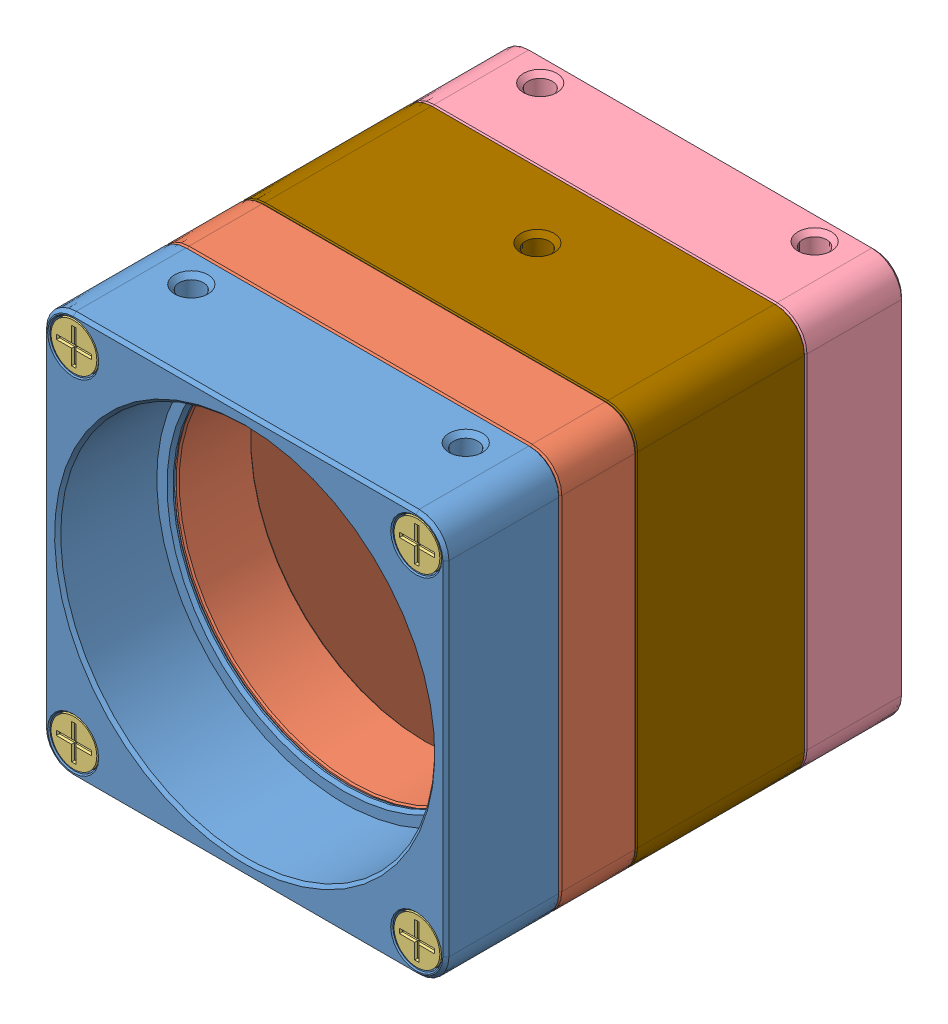
SolidWorks assembly STP-MQ-(MQ022xG-CM)-ASSM, configuration Default. Lengths in mm.
Overall size (26.4 26.4 30.19).
44 component instances, 29 part files, 0 mates.
Components (placement in the parent):
- STP-MQ-(MQ022xG-CM)-ASSM.stp-1: STP-MQ-(MQ022xG-CM)-ASSM.stp [Default] at origin size (26.4 26.4 30.19)
  - SUBASSM-MQ-FRONT.stp-1: SUBASSM-MQ-FRONT.stp [Default] x (0 -1 0) z (0 0 1) size (26.4 26.4 14.6)
    - MECH-MQ-FRONT.stp-1: MECH-MQ-FRONT.stp [Default] at (0 0 7.5) x (1 0 0) z (0 0 -1) size (26.4 26.4 7.5)
    - MECH-MQ-CS-C.stp-1: MECH-MQ-CS-C.stp [Default] at (0 0 0.5) x (1 0 0) z (0 0 -1) size (26.4 26.4 5.5)
    - SROB-M2x14-CUST.stp-1: SROB-M2x14-CUST.stp [Default] at (-11.25 11.25 -7.1) size (3 3 14.55)
    - SROB-M2x14-CUST.stp-2: SROB-M2x14-CUST.stp [Default] at (11.25 -11.25 -7.1) size (3 3 14.55)
    - SROB-M2x14-CUST.stp-3: SROB-M2x14-CUST.stp [Default] at (11.25 11.25 -7.1) size (3 3 14.55)
    - SROB-M2x14-CUST.stp-4: SROB-M2x14-CUST.stp [Default] at (-11.25 -11.25 -7.1) size (3 3 14.55)
  - SUBASSM-MQ-REAR.stp-1: SUBASSM-MQ-REAR.stp [Default] at (0 0 -22.584) x (-1 0 0) z (0 0 1) size (26.4 26.4 10.6)
    - MECH-MQ-REAR.stp-1: MECH-MQ-REAR.stp [Default] at (0 0 6.5) x (-1 0 0) z (0 0 -1) size (26.4 26.4 6.5)
    - SROB-M2x10-CUST .stp-1: SROB-M2x10-CUST .stp [Default] at (-11.25 11.25 10.6) x (1 0 0) z (0 0 -1) size (3 3 10.55)
    - SROB-M2x10-CUST .stp-2: SROB-M2x10-CUST .stp [Default] at (11.25 11.25 10.6) x (1 0 0) z (0 0 -1) size (3 3 10.55)
    - SROB-M2x10-CUST .stp-3: SROB-M2x10-CUST .stp [Default] at (11.25 -11.25 10.6) x (1 0 0) z (0 0 -1) size (3 3 10.55)
    - SROB-M2x10-CUST .stp-4: SROB-M2x10-CUST .stp [Default] at (-11.25 -11.25 10.6) x (1 0 0) z (0 0 -1) size (3 3 10.55)
    - MECH-MQ-THERMAL-PAD.stp-1: MECH-MQ-THERMAL-PAD.stp [Default] at (-10.5 5.45 4.8) x (0.961741 -0.273959 0) z (0 0 -1) size (20.28 8 0.5)
    - MECH-EMI-GSKT-1.3X2.3X11.stp-1: MECH-EMI-GSKT-1.3X2.3X11.stp [Default] at (0 9.9495 3.45) size (11 1.2 3)
    - MECH-EMI-GSKT-1.3X2.3X11.stp-2: MECH-EMI-GSKT-1.3X2.3X11.stp [Default] at (0 7.0505 3.45) size (11 1.2 3)
    - MECH-LIGHTPIPE-1.63X4.14.stp-1: MECH-LIGHTPIPE-1.63X4.14.stp [Default] at (9.3 -3.5 4.1492) x (-1 0 0) z (0 -1 0) size (1.63 4.14 1.63)
    - MECH-LIGHTPIPE-1.63X4.14.stp-2: MECH-LIGHTPIPE-1.63X4.14.stp [Default] at (9.3 -1.5 4.1492) x (-1 0 0) z (0 -1 0) size (1.63 4.14 1.63)
    - MECH-LIGHTPIPE-1.63X4.14.stp-3: MECH-LIGHTPIPE-1.63X4.14.stp [Default] at (9.3 -5.5 4.1492) x (-1 0 0) z (0 -1 0) size (1.63 4.14 1.63)
  - SUBASSM-MQ-MID-022-CM.stp-1: SUBASSM-MQ-MID-022-CM.stp [Default] at (0 0 -4.5) x (-1 0 0) z (0 0 -1) size (26.4 26.4 11.68)
    - MECH-MQ-MID-022-CM-REV2.stp-1: MECH-MQ-MID-022-CM-REV2.stp [Default] at origin size (26.4 26.4 11.59)
    - MECH-O-RING-22X1-VI370.stp-1: MECH-O-RING-22X1-VI370.stp [Default] at (0 0 1.3) x (1 0 0) z (0 1 0) size (24 1 24)
    - FLT-BK7-AR2X-D25.stp-1: FLT-BK7-AR2X-D25.stp [Default] at (0 0 -0.1) size (25 25 1.1)
    - MECH-MX022xG-CM-GSKT.stp-1: MECH-MX022xG-CM-GSKT.stp [Default] at (0 0 3.364) x (0 -1 0) z (0 0 1) size (12.2 17.4 1.27)
  - MQ022xG-CM-PCA-LW_MODEL.stp-1: MQ022xG-CM-PCA-LW_MODEL.stp [Default] at (0 0 -16.486) x (-1 0 0) z (0 0 -1) size (25.43 25.43 13.85)
    - CMV2000.stp-1: CMV2000.stp [Default] at (-0.0259 -0.5261 -1.002) x (-1 0 0) z (0 0 -1) size (18.65 13.5 6.65)
      - ANDON-96UPGA-Socket.stp-1: ANDON-96UPGA-Socket.stp [Default] at origin size (15.9 10.8 3.23)
      - CMV2000_Package.stp-1: CMV2000_Package.stp [Default] at (0 0 3.29) x (-1 0 0) z (0 0 1) size (18.65 13.5 5.45)
      - CMV2000_Glass.stp-1: CMV2000_Glass.stp [Default] at (0 0 6.1) size (18.06 12.95 0.55)
    - MQ022xG-CM-PCA-LW_MODEL-0.stp-1: MQ022xG-CM-PCA-LW_MODEL-0.stp [Default] at origin size (0.25 1.57 4.1)
    - MQ022xG-CM-PCA-LW_MODEL-1.stp-1: MQ022xG-CM-PCA-LW_MODEL-1.stp [Default] at origin size (12.85 2.05 3.8)
    - MQ022xG-CM-PCA-LW_MODEL-2.stp-1: MQ022xG-CM-PCA-LW_MODEL-2.stp [Default] at origin size (25.43 25.43 1)
    - MQ022xG-CM-PCA-LW_MODEL-3.stp-1: MQ022xG-CM-PCA-LW_MODEL-3.stp [Default] at origin size (0.25 1.57 4.1)
    - MQ022xG-CM-PCA-LW_MODEL-4.stp-1: MQ022xG-CM-PCA-LW_MODEL-4.stp [Default] at origin size (5 5 8.1)
    - MQ022xG-CM-PCA-LW_MODEL-5.stp-1: MQ022xG-CM-PCA-LW_MODEL-5.stp [Default] at origin size (0.25 1.57 4.1)
    - MQ022xG-CM-PCA-LW_MODEL-6.stp-1: MQ022xG-CM-PCA-LW_MODEL-6.stp [Default] at origin size (0.25 1.57 4.1)
    - MQ022xG-CM-PCA-LW_MODEL-7.stp-1: MQ022xG-CM-PCA-LW_MODEL-7.stp [Default] at origin size (0.25 1.57 4.1)
    - MQ022xG-CM-PCA-LW_MODEL-8.stp-1: MQ022xG-CM-PCA-LW_MODEL-8.stp [Default] at origin size (0.25 1.57 4.1)
    - MQ022xG-CM-PCA-LW_MODEL-9.stp-1: MQ022xG-CM-PCA-LW_MODEL-9.stp [Default] at origin size (0.25 1.57 4.1)
    - MQ022xG-CM-PCA-LW_MODEL-10.stp-1: MQ022xG-CM-PCA-LW_MODEL-10.stp [Default] at origin size (0.25 1.57 4.1)
    - MQ022xG-CM-PCA-LW_MODEL-11.stp-1: MQ022xG-CM-PCA-LW_MODEL-11.stp [Default] at origin size (0.25 1.57 4.1)
    - MQ022xG-CM-PCA-LW_MODEL-12.stp-1: MQ022xG-CM-PCA-LW_MODEL-12.stp [Default] at origin size (13.8 3 5.6)
    - MQ022xG-CM-PCA-LW_MODEL-13.stp-1: MQ022xG-CM-PCA-LW_MODEL-13.stp [Default] at origin size (0.25 1.57 4.1)
